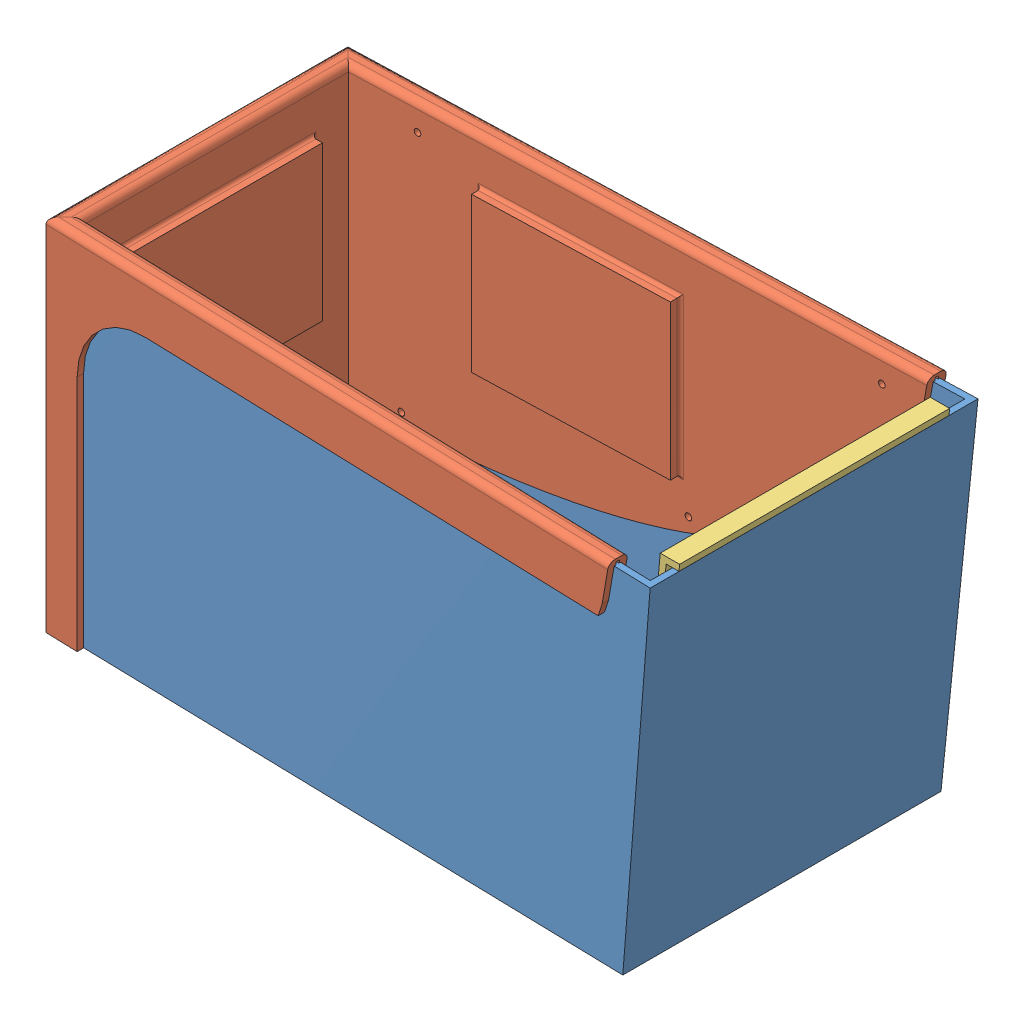
SolidWorks assembly Montagem_cesta_com_SuporteEletronica, configuration Valor predeterminado. Lengths in mm.
Overall size (1005.81 566.86 611.06).
245 component instances, 12 part files, 31 mates.
Components (placement in the parent):
- Cesta_Atualizada-1: Cesta_Atualizada [Valor predeterminado] at (-516.4663 -290.9084 0) size (950 550 510) (hidden)
- SuporteEletronica_Atualizado-1: SuporteEletronica_Atualizado [Valor predeterminado] at (-516.4663 249.0916 0) size (996.8 566.86 611.06)
- SuporteDeEletronica_Tras_Atualizado-1: SuporteDeEletronica_Tras_Atualizado [Valor predeterminado] at (-528.7672 -314.7085 0) size (75.35 498.85 420)
- Antena RFID AN610-2: Antena RFID AN610 [Valor predeterminado] at (-145.1288 78.7469 -224.7205) x (0.999502 0 -0.031563) z (0 -1 0) size (278.3 12.01 216.57)
- Antena RFID AN610-3: Antena RFID AN610 [Valor predeterminado] at (-145.2259 78.7469 224.7174) x (0.999502 0 0.031563) z (0 1 0) size (278.3 12.01 216.57)
- Antena RFID AN610-4: Antena RFID AN610 [Valor predeterminado] at (-504.4663 78.7463 1.4544) x (0 0 1) z (0 1 0) size (278.3 12.01 216.57)
- Antena RFID AN610-6: Antena RFID AN610 [Valor predeterminado] at (399.8873 88.4011 1.4544) x (0 0 1) z (-0.090536 -0.995893 0) size (278.3 12.01 216.57)
- HC-SR04-1: HC-SR04 [Default] at (-534.0577 -216.5172 151.8948) x (0.537325 0 0.843375) z (-0.843375 0 0.537325) size (45.12 25.91 17.5)
  - BoardHCSR04-1: BoardHCSR04 [Default] x (1 0 0) z (0 -1 0) size (45 1.5 20)
  - SOIC16 narrow-1: SOIC16 narrow [Default] at (-18.9903 -0.1332 0.0032) x (0 1 0) z (0 0 -1) size (10.08 6.32 2.01)
  - SOIC16 narrow-2: SOIC16 narrow [Default] at (17.2401 0.0038 0.0032) x (1 0 0) z (0 0 -1) size (10.08 6.32 2.01)
  - SOIC16 narrow-3: SOIC16 narrow [Default] at (0.0833 0.1806 0.0032) x (-1 0 0) z (0 0 -1) size (10.08 6.32 2.01)
  - Crystal Oscillator (SMD)-1: Crystal Oscillator (SMD) [Default] at (0.0865 7.1352 2.4144) x (-1 0 0) z (0 0 1) size (13.06 4.55 4.32)
  - RES 0603-33: RES 0603 [По умолчанию] at (20.0622 -5.1327 -0.45) x (-1 0 0) z (0 1 0) size (1.6 0.45 0.8)
  - RES 0603-30: RES 0603 [По умолчанию] at (20.0876 4.2055 -0.45) x (-1 0 0) z (0 1 0) size (1.6 0.45 0.8)
  - RES 0603-40: RES 0603 [По умолчанию] at (17.1224 8.2736 -0.45) x (-1 0 0) z (0 1 0) size (1.6 0.45 0.8)
  - RES 0603-43: RES 0603 [По умолчанию] at (11.9522 8.2736 -0.45) x (-1 0 0) z (0 1 0) size (1.6 0.45 0.8)
  - RES 0603-44: RES 0603 [По умолчанию] at (14.4328 8.2728 -0.45) x (-1 0 0) z (0 1 0) size (1.6 0.45 0.8)
  - RES 0603-45: RES 0603 [По умолчанию] at (11.4133 -8.8519 -0.45) x (-1 0 0) z (0 1 0) size (1.6 0.45 0.8)
  - RES 0603-46: RES 0603 [По умолчанию] at (9.1337 6.3171 -0.45) x (-1 0 0) z (0 1 0) size (1.6 0.45 0.8)
  - RES 0603-47: RES 0603 [По умолчанию] at (9.131 -5.8347 -0.45) x (-1 0 0) z (0 1 0) size (1.6 0.45 0.8)
  - RES 0603-48: RES 0603 [По умолчанию] at (9.1319 -3.7587 -0.45) x (-1 0 0) z (0 1 0) size (1.6 0.45 0.8)
  - RES 0603-49: RES 0603 [По умолчанию] at (9.1326 -1.7712 -0.45) x (-1 0 0) z (0 1 0) size (1.6 0.45 0.8)
  - RES 0603-50: RES 0603 [По умолчанию] at (-8.574 5.1664 -0.45) x (-1 0 0) z (0 1 0) size (1.6 0.45 0.8)
  - RES 0603-51: RES 0603 [По умолчанию] at (-8.6599 1.0553 -0.45) x (-1 0 0) z (0 1 0) size (1.6 0.45 0.8)
  - RES 0603-52: RES 0603 [По умолчанию] at (-8.6597 -0.8895 -0.45) x (-1 0 0) z (0 1 0) size (1.6 0.45 0.8)
  - RES 0603-53: RES 0603 [По умолчанию] at (-8.6224 -2.9356 -0.45) x (-1 0 0) z (0 1 0) size (1.6 0.45 0.8)
  - RES 0603-54: RES 0603 [По умолчанию] at (-8.6219 -5.2391 -0.45) x (-1 0 0) z (0 1 0) size (1.6 0.45 0.8)
  - RES 0603-55: RES 0603 [По умолчанию] at (-18.792 -7.4397 -0.45) x (-1 0 0) z (0 1 0) size (1.6 0.45 0.8)
  - RES 0603-56: RES 0603 [По умолчанию] at (-18.792 6.206 -0.45) x (-1 0 0) z (0 1 0) size (1.6 0.45 0.8)
  - 0603 Capacitor-2: 0603 Capacitor [Default] at (18.0116 -4.5871 0) x (0 -1 0) z (0 0 -1) size (1.6 0.84 0.84)
  - 0603 Capacitor-7: 0603 Capacitor [Default] at (15.4963 -8.9009 0) x (-1 0 0) z (0 0 -1) size (1.6 0.84 0.84)
  - 0603 Capacitor-8: 0603 Capacitor [Default] at (9.8433 0.2097 0) x (-1 0 0) z (0 0 -1) size (1.6 0.84 0.84)
  - 0603 Capacitor-17: 0603 Capacitor [Default] at (-7.8216 3.0281 0) x (-1 0 0) z (0 0 -1) size (1.6 0.84 0.84)
  - 0603 Capacitor-18: 0603 Capacitor [Default] at (18.0081 6.1516 0) x (0 -1 0) z (0 0 -1) size (1.6 0.84 0.84)
  - 0603 Capacitor-19: 0603 Capacitor [Default] at (9.8432 2.0135 0) x (-1 0 0) z (0 0 -1) size (1.6 0.84 0.84)
  - 0603 Capacitor-22: 0603 Capacitor [Default] at (9.843 3.9787 0) x (-1 0 0) z (0 0 -1) size (1.6 0.84 0.84)
  - Mesh-1: Mesh [Default] at (-7.5462 11.7833 1.7797) x (-0.435927 -0.899982 0) z (0 0 -1) size (13.88 13.88 0.41)
  - Mesh-2: Mesh [Default] at (5.988 10.9085 24.5426) x (0.558295 -0.829642 0) z (0 0 1) size (13.88 13.88 0.41)
  - PLS-4R (DS-1022-1x4)-1: PLS-4R (DS-1022-1x4) [another] at (3.81 -8.73 -2.5) x (0 -1 0) z (-1 0 0) size (8.45 7 10.16)
  - Transmitter-1: Transmitter [Default] at (0 0 1.5) x (-1 0 0) z (0 0 -1) size (42 16 14.5)
- HC-SR04-2: HC-SR04 [Default] at (-545.4669 -216.5172 115.0138) x (0.066401 0 0.997793) z (-0.997793 0 0.066401) size (45.12 25.91 17.5)
  - BoardHCSR04-1: BoardHCSR04 [Default] x (1 0 0) z (0 -1 0) size (45 1.5 20)
  - SOIC16 narrow-1: SOIC16 narrow [Default] at (-18.9903 -0.1332 0.0032) x (0 1 0) z (0 0 -1) size (10.08 6.32 2.01)
  - SOIC16 narrow-2: SOIC16 narrow [Default] at (17.2401 0.0038 0.0032) x (1 0 0) z (0 0 -1) size (10.08 6.32 2.01)
  - SOIC16 narrow-3: SOIC16 narrow [Default] at (0.0833 0.1806 0.0032) x (-1 0 0) z (0 0 -1) size (10.08 6.32 2.01)
  - Crystal Oscillator (SMD)-1: Crystal Oscillator (SMD) [Default] at (0.0865 7.1352 2.4144) x (-1 0 0) z (0 0 1) size (13.06 4.55 4.32)
  - RES 0603-33: RES 0603 [По умолчанию] at (20.0622 -5.1327 -0.45) x (-1 0 0) z (0 1 0) size (1.6 0.45 0.8)
  - RES 0603-30: RES 0603 [По умолчанию] at (20.0876 4.2055 -0.45) x (-1 0 0) z (0 1 0) size (1.6 0.45 0.8)
  - RES 0603-40: RES 0603 [По умолчанию] at (17.1224 8.2736 -0.45) x (-1 0 0) z (0 1 0) size (1.6 0.45 0.8)
  - RES 0603-43: RES 0603 [По умолчанию] at (11.9522 8.2736 -0.45) x (-1 0 0) z (0 1 0) size (1.6 0.45 0.8)
  - RES 0603-44: RES 0603 [По умолчанию] at (14.4328 8.2728 -0.45) x (-1 0 0) z (0 1 0) size (1.6 0.45 0.8)
  - RES 0603-45: RES 0603 [По умолчанию] at (11.4133 -8.8519 -0.45) x (-1 0 0) z (0 1 0) size (1.6 0.45 0.8)
  - RES 0603-46: RES 0603 [По умолчанию] at (9.1337 6.3171 -0.45) x (-1 0 0) z (0 1 0) size (1.6 0.45 0.8)
  - RES 0603-47: RES 0603 [По умолчанию] at (9.131 -5.8347 -0.45) x (-1 0 0) z (0 1 0) size (1.6 0.45 0.8)
  - RES 0603-48: RES 0603 [По умолчанию] at (9.1319 -3.7587 -0.45) x (-1 0 0) z (0 1 0) size (1.6 0.45 0.8)
  - RES 0603-49: RES 0603 [По умолчанию] at (9.1326 -1.7712 -0.45) x (-1 0 0) z (0 1 0) size (1.6 0.45 0.8)
  - RES 0603-50: RES 0603 [По умолчанию] at (-8.574 5.1664 -0.45) x (-1 0 0) z (0 1 0) size (1.6 0.45 0.8)
  - RES 0603-51: RES 0603 [По умолчанию] at (-8.6599 1.0553 -0.45) x (-1 0 0) z (0 1 0) size (1.6 0.45 0.8)
  - RES 0603-52: RES 0603 [По умолчанию] at (-8.6597 -0.8895 -0.45) x (-1 0 0) z (0 1 0) size (1.6 0.45 0.8)
  - RES 0603-53: RES 0603 [По умолчанию] at (-8.6224 -2.9356 -0.45) x (-1 0 0) z (0 1 0) size (1.6 0.45 0.8)
  - RES 0603-54: RES 0603 [По умолчанию] at (-8.6219 -5.2391 -0.45) x (-1 0 0) z (0 1 0) size (1.6 0.45 0.8)
  - RES 0603-55: RES 0603 [По умолчанию] at (-18.792 -7.4397 -0.45) x (-1 0 0) z (0 1 0) size (1.6 0.45 0.8)
  - RES 0603-56: RES 0603 [По умолчанию] at (-18.792 6.206 -0.45) x (-1 0 0) z (0 1 0) size (1.6 0.45 0.8)
  - 0603 Capacitor-2: 0603 Capacitor [Default] at (18.0116 -4.5871 0) x (0 -1 0) z (0 0 -1) size (1.6 0.84 0.84)
  - 0603 Capacitor-7: 0603 Capacitor [Default] at (15.4963 -8.9009 0) x (-1 0 0) z (0 0 -1) size (1.6 0.84 0.84)
  - 0603 Capacitor-8: 0603 Capacitor [Default] at (9.8433 0.2097 0) x (-1 0 0) z (0 0 -1) size (1.6 0.84 0.84)
  - 0603 Capacitor-17: 0603 Capacitor [Default] at (-7.8216 3.0281 0) x (-1 0 0) z (0 0 -1) size (1.6 0.84 0.84)
  - 0603 Capacitor-18: 0603 Capacitor [Default] at (18.0081 6.1516 0) x (0 -1 0) z (0 0 -1) size (1.6 0.84 0.84)
  - 0603 Capacitor-19: 0603 Capacitor [Default] at (9.8432 2.0135 0) x (-1 0 0) z (0 0 -1) size (1.6 0.84 0.84)
  - 0603 Capacitor-22: 0603 Capacitor [Default] at (9.843 3.9787 0) x (-1 0 0) z (0 0 -1) size (1.6 0.84 0.84)
  - Mesh-1: Mesh [Default] at (-7.5462 11.7833 1.7797) x (-0.435927 -0.899982 0) z (0 0 -1) size (13.88 13.88 0.41)
  - Mesh-2: Mesh [Default] at (5.988 10.9085 24.5426) x (0.558295 -0.829642 0) z (0 0 1) size (13.88 13.88 0.41)
  - PLS-4R (DS-1022-1x4)-1: PLS-4R (DS-1022-1x4) [another] at (3.81 -8.73 -2.5) x (0 -1 0) z (-1 0 0) size (8.45 7 10.16)
  - Transmitter-1: Transmitter [Default] at (0 0 1.5) x (-1 0 0) z (0 0 -1) size (42 16 14.5)
- HC-SR04-3: HC-SR04 [Default] at (-549.4828 -216.5172 57.0525) x (0.071003 0 0.997476) z (-0.997476 0 0.071003) size (45.12 25.91 17.5)
  - BoardHCSR04-1: BoardHCSR04 [Default] x (1 0 0) z (0 -1 0) size (45 1.5 20)
  - SOIC16 narrow-1: SOIC16 narrow [Default] at (-18.9903 -0.1332 0.0032) x (0 1 0) z (0 0 -1) size (10.08 6.32 2.01)
  - SOIC16 narrow-2: SOIC16 narrow [Default] at (17.2401 0.0038 0.0032) x (1 0 0) z (0 0 -1) size (10.08 6.32 2.01)
  - SOIC16 narrow-3: SOIC16 narrow [Default] at (0.0833 0.1806 0.0032) x (-1 0 0) z (0 0 -1) size (10.08 6.32 2.01)
  - Crystal Oscillator (SMD)-1: Crystal Oscillator (SMD) [Default] at (0.0865 7.1352 2.4144) x (-1 0 0) z (0 0 1) size (13.06 4.55 4.32)
  - RES 0603-33: RES 0603 [По умолчанию] at (20.0622 -5.1327 -0.45) x (-1 0 0) z (0 1 0) size (1.6 0.45 0.8)
  - RES 0603-30: RES 0603 [По умолчанию] at (20.0876 4.2055 -0.45) x (-1 0 0) z (0 1 0) size (1.6 0.45 0.8)
  - RES 0603-40: RES 0603 [По умолчанию] at (17.1224 8.2736 -0.45) x (-1 0 0) z (0 1 0) size (1.6 0.45 0.8)
  - RES 0603-43: RES 0603 [По умолчанию] at (11.9522 8.2736 -0.45) x (-1 0 0) z (0 1 0) size (1.6 0.45 0.8)
  - RES 0603-44: RES 0603 [По умолчанию] at (14.4328 8.2728 -0.45) x (-1 0 0) z (0 1 0) size (1.6 0.45 0.8)
  - RES 0603-45: RES 0603 [По умолчанию] at (11.4133 -8.8519 -0.45) x (-1 0 0) z (0 1 0) size (1.6 0.45 0.8)
  - RES 0603-46: RES 0603 [По умолчанию] at (9.1337 6.3171 -0.45) x (-1 0 0) z (0 1 0) size (1.6 0.45 0.8)
  - RES 0603-47: RES 0603 [По умолчанию] at (9.131 -5.8347 -0.45) x (-1 0 0) z (0 1 0) size (1.6 0.45 0.8)
  - RES 0603-48: RES 0603 [По умолчанию] at (9.1319 -3.7587 -0.45) x (-1 0 0) z (0 1 0) size (1.6 0.45 0.8)
  - RES 0603-49: RES 0603 [По умолчанию] at (9.1326 -1.7712 -0.45) x (-1 0 0) z (0 1 0) size (1.6 0.45 0.8)
  - RES 0603-50: RES 0603 [По умолчанию] at (-8.574 5.1664 -0.45) x (-1 0 0) z (0 1 0) size (1.6 0.45 0.8)
  - RES 0603-51: RES 0603 [По умолчанию] at (-8.6599 1.0553 -0.45) x (-1 0 0) z (0 1 0) size (1.6 0.45 0.8)
  - RES 0603-52: RES 0603 [По умолчанию] at (-8.6597 -0.8895 -0.45) x (-1 0 0) z (0 1 0) size (1.6 0.45 0.8)
  - RES 0603-53: RES 0603 [По умолчанию] at (-8.6224 -2.9356 -0.45) x (-1 0 0) z (0 1 0) size (1.6 0.45 0.8)
  - RES 0603-54: RES 0603 [По умолчанию] at (-8.6219 -5.2391 -0.45) x (-1 0 0) z (0 1 0) size (1.6 0.45 0.8)
  - RES 0603-55: RES 0603 [По умолчанию] at (-18.792 -7.4397 -0.45) x (-1 0 0) z (0 1 0) size (1.6 0.45 0.8)
  - RES 0603-56: RES 0603 [По умолчанию] at (-18.792 6.206 -0.45) x (-1 0 0) z (0 1 0) size (1.6 0.45 0.8)
  - 0603 Capacitor-2: 0603 Capacitor [Default] at (18.0116 -4.5871 0) x (0 -1 0) z (0 0 -1) size (1.6 0.84 0.84)
  - 0603 Capacitor-7: 0603 Capacitor [Default] at (15.4963 -8.9009 0) x (-1 0 0) z (0 0 -1) size (1.6 0.84 0.84)
  - 0603 Capacitor-8: 0603 Capacitor [Default] at (9.8433 0.2097 0) x (-1 0 0) z (0 0 -1) size (1.6 0.84 0.84)
  - 0603 Capacitor-17: 0603 Capacitor [Default] at (-7.8216 3.0281 0) x (-1 0 0) z (0 0 -1) size (1.6 0.84 0.84)
  - 0603 Capacitor-18: 0603 Capacitor [Default] at (18.0081 6.1516 0) x (0 -1 0) z (0 0 -1) size (1.6 0.84 0.84)
  - 0603 Capacitor-19: 0603 Capacitor [Default] at (9.8432 2.0135 0) x (-1 0 0) z (0 0 -1) size (1.6 0.84 0.84)
  - 0603 Capacitor-22: 0603 Capacitor [Default] at (9.843 3.9787 0) x (-1 0 0) z (0 0 -1) size (1.6 0.84 0.84)
  - Mesh-1: Mesh [Default] at (-7.5462 11.7833 1.7797) x (-0.435927 -0.899982 0) z (0 0 -1) size (13.88 13.88 0.41)
  - Mesh-2: Mesh [Default] at (5.988 10.9085 24.5426) x (0.558295 -0.829642 0) z (0 0 1) size (13.88 13.88 0.41)
  - PLS-4R (DS-1022-1x4)-1: PLS-4R (DS-1022-1x4) [another] at (3.81 -8.73 -2.5) x (0 -1 0) z (-1 0 0) size (8.45 7 10.16)
  - Transmitter-1: Transmitter [Default] at (0 0 1.5) x (-1 0 0) z (0 0 -1) size (42 16 14.5)
- HC-SR04-4: HC-SR04 [Default] at (-551.8136 -216.5172 -0.4786) x (0 0 1) z (-1 0 0) size (45.12 25.91 17.5)
  - BoardHCSR04-1: BoardHCSR04 [Default] x (1 0 0) z (0 -1 0) size (45 1.5 20)
  - SOIC16 narrow-1: SOIC16 narrow [Default] at (-18.9903 -0.1332 0.0032) x (0 1 0) z (0 0 -1) size (10.08 6.32 2.01)
  - SOIC16 narrow-2: SOIC16 narrow [Default] at (17.2401 0.0038 0.0032) x (1 0 0) z (0 0 -1) size (10.08 6.32 2.01)
  - SOIC16 narrow-3: SOIC16 narrow [Default] at (0.0833 0.1806 0.0032) x (-1 0 0) z (0 0 -1) size (10.08 6.32 2.01)
  - Crystal Oscillator (SMD)-1: Crystal Oscillator (SMD) [Default] at (0.0865 7.1352 2.4144) x (-1 0 0) z (0 0 1) size (13.06 4.55 4.32)
  - RES 0603-33: RES 0603 [По умолчанию] at (20.0622 -5.1327 -0.45) x (-1 0 0) z (0 1 0) size (1.6 0.45 0.8)
  - RES 0603-30: RES 0603 [По умолчанию] at (20.0876 4.2055 -0.45) x (-1 0 0) z (0 1 0) size (1.6 0.45 0.8)
  - RES 0603-40: RES 0603 [По умолчанию] at (17.1224 8.2736 -0.45) x (-1 0 0) z (0 1 0) size (1.6 0.45 0.8)
  - RES 0603-43: RES 0603 [По умолчанию] at (11.9522 8.2736 -0.45) x (-1 0 0) z (0 1 0) size (1.6 0.45 0.8)
  - RES 0603-44: RES 0603 [По умолчанию] at (14.4328 8.2728 -0.45) x (-1 0 0) z (0 1 0) size (1.6 0.45 0.8)
  - RES 0603-45: RES 0603 [По умолчанию] at (11.4133 -8.8519 -0.45) x (-1 0 0) z (0 1 0) size (1.6 0.45 0.8)
  - RES 0603-46: RES 0603 [По умолчанию] at (9.1337 6.3171 -0.45) x (-1 0 0) z (0 1 0) size (1.6 0.45 0.8)
  - RES 0603-47: RES 0603 [По умолчанию] at (9.131 -5.8347 -0.45) x (-1 0 0) z (0 1 0) size (1.6 0.45 0.8)
  - RES 0603-48: RES 0603 [По умолчанию] at (9.1319 -3.7587 -0.45) x (-1 0 0) z (0 1 0) size (1.6 0.45 0.8)
  - RES 0603-49: RES 0603 [По умолчанию] at (9.1326 -1.7712 -0.45) x (-1 0 0) z (0 1 0) size (1.6 0.45 0.8)
  - RES 0603-50: RES 0603 [По умолчанию] at (-8.574 5.1664 -0.45) x (-1 0 0) z (0 1 0) size (1.6 0.45 0.8)
  - RES 0603-51: RES 0603 [По умолчанию] at (-8.6599 1.0553 -0.45) x (-1 0 0) z (0 1 0) size (1.6 0.45 0.8)
  - RES 0603-52: RES 0603 [По умолчанию] at (-8.6597 -0.8895 -0.45) x (-1 0 0) z (0 1 0) size (1.6 0.45 0.8)
  - RES 0603-53: RES 0603 [По умолчанию] at (-8.6224 -2.9356 -0.45) x (-1 0 0) z (0 1 0) size (1.6 0.45 0.8)
  - RES 0603-54: RES 0603 [По умолчанию] at (-8.6219 -5.2391 -0.45) x (-1 0 0) z (0 1 0) size (1.6 0.45 0.8)
  - RES 0603-55: RES 0603 [По умолчанию] at (-18.792 -7.4397 -0.45) x (-1 0 0) z (0 1 0) size (1.6 0.45 0.8)
  - RES 0603-56: RES 0603 [По умолчанию] at (-18.792 6.206 -0.45) x (-1 0 0) z (0 1 0) size (1.6 0.45 0.8)
  - 0603 Capacitor-2: 0603 Capacitor [Default] at (18.0116 -4.5871 0) x (0 -1 0) z (0 0 -1) size (1.6 0.84 0.84)
  - 0603 Capacitor-7: 0603 Capacitor [Default] at (15.4963 -8.9009 0) x (-1 0 0) z (0 0 -1) size (1.6 0.84 0.84)
  - 0603 Capacitor-8: 0603 Capacitor [Default] at (9.8433 0.2097 0) x (-1 0 0) z (0 0 -1) size (1.6 0.84 0.84)
  - 0603 Capacitor-17: 0603 Capacitor [Default] at (-7.8216 3.0281 0) x (-1 0 0) z (0 0 -1) size (1.6 0.84 0.84)
  - 0603 Capacitor-18: 0603 Capacitor [Default] at (18.0081 6.1516 0) x (0 -1 0) z (0 0 -1) size (1.6 0.84 0.84)
  - 0603 Capacitor-19: 0603 Capacitor [Default] at (9.8432 2.0135 0) x (-1 0 0) z (0 0 -1) size (1.6 0.84 0.84)
  - 0603 Capacitor-22: 0603 Capacitor [Default] at (9.843 3.9787 0) x (-1 0 0) z (0 0 -1) size (1.6 0.84 0.84)
  - Mesh-1: Mesh [Default] at (-7.5462 11.7833 1.7797) x (-0.435927 -0.899982 0) z (0 0 -1) size (13.88 13.88 0.41)
  - Mesh-2: Mesh [Default] at (5.988 10.9085 24.5426) x (0.558295 -0.829642 0) z (0 0 1) size (13.88 13.88 0.41)
  - PLS-4R (DS-1022-1x4)-1: PLS-4R (DS-1022-1x4) [another] at (3.81 -8.73 -2.5) x (0 -1 0) z (-1 0 0) size (8.45 7 10.16)
  - Transmitter-1: Transmitter [Default] at (0 0 1.5) x (-1 0 0) z (0 0 -1) size (42 16 14.5)
- HC-SR04-5: HC-SR04 [Default] at (-549.4139 -216.5172 -58.0073) x (-0.071003 0 0.997476) z (-0.997476 0 -0.071003) size (45.12 25.91 17.5)
  - BoardHCSR04-1: BoardHCSR04 [Default] x (1 0 0) z (0 -1 0) size (45 1.5 20)
  - SOIC16 narrow-1: SOIC16 narrow [Default] at (-18.9903 -0.1332 0.0032) x (0 1 0) z (0 0 -1) size (10.08 6.32 2.01)
  - SOIC16 narrow-2: SOIC16 narrow [Default] at (17.2401 0.0038 0.0032) x (1 0 0) z (0 0 -1) size (10.08 6.32 2.01)
  - SOIC16 narrow-3: SOIC16 narrow [Default] at (0.0833 0.1806 0.0032) x (-1 0 0) z (0 0 -1) size (10.08 6.32 2.01)
  - Crystal Oscillator (SMD)-1: Crystal Oscillator (SMD) [Default] at (0.0865 7.1352 2.4144) x (-1 0 0) z (0 0 1) size (13.06 4.55 4.32)
  - RES 0603-33: RES 0603 [По умолчанию] at (20.0622 -5.1327 -0.45) x (-1 0 0) z (0 1 0) size (1.6 0.45 0.8)
  - RES 0603-30: RES 0603 [По умолчанию] at (20.0876 4.2055 -0.45) x (-1 0 0) z (0 1 0) size (1.6 0.45 0.8)
  - RES 0603-40: RES 0603 [По умолчанию] at (17.1224 8.2736 -0.45) x (-1 0 0) z (0 1 0) size (1.6 0.45 0.8)
  - RES 0603-43: RES 0603 [По умолчанию] at (11.9522 8.2736 -0.45) x (-1 0 0) z (0 1 0) size (1.6 0.45 0.8)
  - RES 0603-44: RES 0603 [По умолчанию] at (14.4328 8.2728 -0.45) x (-1 0 0) z (0 1 0) size (1.6 0.45 0.8)
  - RES 0603-45: RES 0603 [По умолчанию] at (11.4133 -8.8519 -0.45) x (-1 0 0) z (0 1 0) size (1.6 0.45 0.8)
  - RES 0603-46: RES 0603 [По умолчанию] at (9.1337 6.3171 -0.45) x (-1 0 0) z (0 1 0) size (1.6 0.45 0.8)
  - RES 0603-47: RES 0603 [По умолчанию] at (9.131 -5.8347 -0.45) x (-1 0 0) z (0 1 0) size (1.6 0.45 0.8)
  - RES 0603-48: RES 0603 [По умолчанию] at (9.1319 -3.7587 -0.45) x (-1 0 0) z (0 1 0) size (1.6 0.45 0.8)
  - RES 0603-49: RES 0603 [По умолчанию] at (9.1326 -1.7712 -0.45) x (-1 0 0) z (0 1 0) size (1.6 0.45 0.8)
  - RES 0603-50: RES 0603 [По умолчанию] at (-8.574 5.1664 -0.45) x (-1 0 0) z (0 1 0) size (1.6 0.45 0.8)
  - RES 0603-51: RES 0603 [По умолчанию] at (-8.6599 1.0553 -0.45) x (-1 0 0) z (0 1 0) size (1.6 0.45 0.8)
  - RES 0603-52: RES 0603 [По умолчанию] at (-8.6597 -0.8895 -0.45) x (-1 0 0) z (0 1 0) size (1.6 0.45 0.8)
  - RES 0603-53: RES 0603 [По умолчанию] at (-8.6224 -2.9356 -0.45) x (-1 0 0) z (0 1 0) size (1.6 0.45 0.8)
  - RES 0603-54: RES 0603 [По умолчанию] at (-8.6219 -5.2391 -0.45) x (-1 0 0) z (0 1 0) size (1.6 0.45 0.8)
  - RES 0603-55: RES 0603 [По умолчанию] at (-18.792 -7.4397 -0.45) x (-1 0 0) z (0 1 0) size (1.6 0.45 0.8)
  - RES 0603-56: RES 0603 [По умолчанию] at (-18.792 6.206 -0.45) x (-1 0 0) z (0 1 0) size (1.6 0.45 0.8)
  - 0603 Capacitor-2: 0603 Capacitor [Default] at (18.0116 -4.5871 0) x (0 -1 0) z (0 0 -1) size (1.6 0.84 0.84)
  - 0603 Capacitor-7: 0603 Capacitor [Default] at (15.4963 -8.9009 0) x (-1 0 0) z (0 0 -1) size (1.6 0.84 0.84)
  - 0603 Capacitor-8: 0603 Capacitor [Default] at (9.8433 0.2097 0) x (-1 0 0) z (0 0 -1) size (1.6 0.84 0.84)
  - 0603 Capacitor-17: 0603 Capacitor [Default] at (-7.8216 3.0281 0) x (-1 0 0) z (0 0 -1) size (1.6 0.84 0.84)
  - 0603 Capacitor-18: 0603 Capacitor [Default] at (18.0081 6.1516 0) x (0 -1 0) z (0 0 -1) size (1.6 0.84 0.84)
  - 0603 Capacitor-19: 0603 Capacitor [Default] at (9.8432 2.0135 0) x (-1 0 0) z (0 0 -1) size (1.6 0.84 0.84)
  - 0603 Capacitor-22: 0603 Capacitor [Default] at (9.843 3.9787 0) x (-1 0 0) z (0 0 -1) size (1.6 0.84 0.84)
  - Mesh-1: Mesh [Default] at (-7.5462 11.7833 1.7797) x (-0.435927 -0.899982 0) z (0 0 -1) size (13.88 13.88 0.41)
  - Mesh-2: Mesh [Default] at (5.988 10.9085 24.5426) x (0.558295 -0.829642 0) z (0 0 1) size (13.88 13.88 0.41)
  - PLS-4R (DS-1022-1x4)-1: PLS-4R (DS-1022-1x4) [another] at (3.81 -8.73 -2.5) x (0 -1 0) z (-1 0 0) size (8.45 7 10.16)
  - Transmitter-1: Transmitter [Default] at (0 0 1.5) x (-1 0 0) z (0 0 -1) size (42 16 14.5)
- HC-SR04-6: HC-SR04 [Default] at (-545.3183 -216.5172 -117.2336) x (-0.066401 0 0.997793) z (-0.997793 0 -0.066401) size (45.12 25.91 17.5)
  - BoardHCSR04-1: BoardHCSR04 [Default] x (1 0 0) z (0 -1 0) size (45 1.5 20)
  - SOIC16 narrow-1: SOIC16 narrow [Default] at (-18.9903 -0.1332 0.0032) x (0 1 0) z (0 0 -1) size (10.08 6.32 2.01)
  - SOIC16 narrow-2: SOIC16 narrow [Default] at (17.2401 0.0038 0.0032) x (1 0 0) z (0 0 -1) size (10.08 6.32 2.01)
  - SOIC16 narrow-3: SOIC16 narrow [Default] at (0.0833 0.1806 0.0032) x (-1 0 0) z (0 0 -1) size (10.08 6.32 2.01)
  - Crystal Oscillator (SMD)-1: Crystal Oscillator (SMD) [Default] at (0.0865 7.1352 2.4144) x (-1 0 0) z (0 0 1) size (13.06 4.55 4.32)
  - RES 0603-33: RES 0603 [По умолчанию] at (20.0622 -5.1327 -0.45) x (-1 0 0) z (0 1 0) size (1.6 0.45 0.8)
  - RES 0603-30: RES 0603 [По умолчанию] at (20.0876 4.2055 -0.45) x (-1 0 0) z (0 1 0) size (1.6 0.45 0.8)
  - RES 0603-40: RES 0603 [По умолчанию] at (17.1224 8.2736 -0.45) x (-1 0 0) z (0 1 0) size (1.6 0.45 0.8)
  - RES 0603-43: RES 0603 [По умолчанию] at (11.9522 8.2736 -0.45) x (-1 0 0) z (0 1 0) size (1.6 0.45 0.8)
  - RES 0603-44: RES 0603 [По умолчанию] at (14.4328 8.2728 -0.45) x (-1 0 0) z (0 1 0) size (1.6 0.45 0.8)
  - RES 0603-45: RES 0603 [По умолчанию] at (11.4133 -8.8519 -0.45) x (-1 0 0) z (0 1 0) size (1.6 0.45 0.8)
  - RES 0603-46: RES 0603 [По умолчанию] at (9.1337 6.3171 -0.45) x (-1 0 0) z (0 1 0) size (1.6 0.45 0.8)
  - RES 0603-47: RES 0603 [По умолчанию] at (9.131 -5.8347 -0.45) x (-1 0 0) z (0 1 0) size (1.6 0.45 0.8)
  - RES 0603-48: RES 0603 [По умолчанию] at (9.1319 -3.7587 -0.45) x (-1 0 0) z (0 1 0) size (1.6 0.45 0.8)
  - RES 0603-49: RES 0603 [По умолчанию] at (9.1326 -1.7712 -0.45) x (-1 0 0) z (0 1 0) size (1.6 0.45 0.8)
  - RES 0603-50: RES 0603 [По умолчанию] at (-8.574 5.1664 -0.45) x (-1 0 0) z (0 1 0) size (1.6 0.45 0.8)
  - RES 0603-51: RES 0603 [По умолчанию] at (-8.6599 1.0553 -0.45) x (-1 0 0) z (0 1 0) size (1.6 0.45 0.8)
  - RES 0603-52: RES 0603 [По умолчанию] at (-8.6597 -0.8895 -0.45) x (-1 0 0) z (0 1 0) size (1.6 0.45 0.8)
  - RES 0603-53: RES 0603 [По умолчанию] at (-8.6224 -2.9356 -0.45) x (-1 0 0) z (0 1 0) size (1.6 0.45 0.8)
  - RES 0603-54: RES 0603 [По умолчанию] at (-8.6219 -5.2391 -0.45) x (-1 0 0) z (0 1 0) size (1.6 0.45 0.8)
  - RES 0603-55: RES 0603 [По умолчанию] at (-18.792 -7.4397 -0.45) x (-1 0 0) z (0 1 0) size (1.6 0.45 0.8)
  - RES 0603-56: RES 0603 [По умолчанию] at (-18.792 6.206 -0.45) x (-1 0 0) z (0 1 0) size (1.6 0.45 0.8)
  - 0603 Capacitor-2: 0603 Capacitor [Default] at (18.0116 -4.5871 0) x (0 -1 0) z (0 0 -1) size (1.6 0.84 0.84)
  - 0603 Capacitor-7: 0603 Capacitor [Default] at (15.4963 -8.9009 0) x (-1 0 0) z (0 0 -1) size (1.6 0.84 0.84)
  - 0603 Capacitor-8: 0603 Capacitor [Default] at (9.8433 0.2097 0) x (-1 0 0) z (0 0 -1) size (1.6 0.84 0.84)
  - 0603 Capacitor-17: 0603 Capacitor [Default] at (-7.8216 3.0281 0) x (-1 0 0) z (0 0 -1) size (1.6 0.84 0.84)
  - 0603 Capacitor-18: 0603 Capacitor [Default] at (18.0081 6.1516 0) x (0 -1 0) z (0 0 -1) size (1.6 0.84 0.84)
  - 0603 Capacitor-19: 0603 Capacitor [Default] at (9.8432 2.0135 0) x (-1 0 0) z (0 0 -1) size (1.6 0.84 0.84)
  - 0603 Capacitor-22: 0603 Capacitor [Default] at (9.843 3.9787 0) x (-1 0 0) z (0 0 -1) size (1.6 0.84 0.84)
  - Mesh-1: Mesh [Default] at (-7.5462 11.7833 1.7797) x (-0.435927 -0.899982 0) z (0 0 -1) size (13.88 13.88 0.41)
  - Mesh-2: Mesh [Default] at (5.988 10.9085 24.5426) x (0.558295 -0.829642 0) z (0 0 1) size (13.88 13.88 0.41)
  - PLS-4R (DS-1022-1x4)-1: PLS-4R (DS-1022-1x4) [another] at (3.81 -8.73 -2.5) x (0 -1 0) z (-1 0 0) size (8.45 7 10.16)
  - Transmitter-1: Transmitter [Default] at (0 0 1.5) x (-1 0 0) z (0 0 -1) size (42 16 14.5)
- HC-SR04-7: HC-SR04 [Default] at (-532.8551 -216.5172 -153.7689) x (-0.537325 0 0.843375) z (-0.843375 0 -0.537325) size (45.12 25.91 17.5)
  - BoardHCSR04-1: BoardHCSR04 [Default] x (1 0 0) z (0 -1 0) size (45 1.5 20)
  - SOIC16 narrow-1: SOIC16 narrow [Default] at (-18.9903 -0.1332 0.0032) x (0 1 0) z (0 0 -1) size (10.08 6.32 2.01)
  - SOIC16 narrow-2: SOIC16 narrow [Default] at (17.2401 0.0038 0.0032) x (1 0 0) z (0 0 -1) size (10.08 6.32 2.01)
  - SOIC16 narrow-3: SOIC16 narrow [Default] at (0.0833 0.1806 0.0032) x (-1 0 0) z (0 0 -1) size (10.08 6.32 2.01)
  - Crystal Oscillator (SMD)-1: Crystal Oscillator (SMD) [Default] at (0.0865 7.1352 2.4144) x (-1 0 0) z (0 0 1) size (13.06 4.55 4.32)
  - RES 0603-33: RES 0603 [По умолчанию] at (20.0622 -5.1327 -0.45) x (-1 0 0) z (0 1 0) size (1.6 0.45 0.8)
  - RES 0603-30: RES 0603 [По умолчанию] at (20.0876 4.2055 -0.45) x (-1 0 0) z (0 1 0) size (1.6 0.45 0.8)
  - RES 0603-40: RES 0603 [По умолчанию] at (17.1224 8.2736 -0.45) x (-1 0 0) z (0 1 0) size (1.6 0.45 0.8)
  - RES 0603-43: RES 0603 [По умолчанию] at (11.9522 8.2736 -0.45) x (-1 0 0) z (0 1 0) size (1.6 0.45 0.8)
  - RES 0603-44: RES 0603 [По умолчанию] at (14.4328 8.2728 -0.45) x (-1 0 0) z (0 1 0) size (1.6 0.45 0.8)
  - RES 0603-45: RES 0603 [По умолчанию] at (11.4133 -8.8519 -0.45) x (-1 0 0) z (0 1 0) size (1.6 0.45 0.8)
  - RES 0603-46: RES 0603 [По умолчанию] at (9.1337 6.3171 -0.45) x (-1 0 0) z (0 1 0) size (1.6 0.45 0.8)
  - RES 0603-47: RES 0603 [По умолчанию] at (9.131 -5.8347 -0.45) x (-1 0 0) z (0 1 0) size (1.6 0.45 0.8)
  - RES 0603-48: RES 0603 [По умолчанию] at (9.1319 -3.7587 -0.45) x (-1 0 0) z (0 1 0) size (1.6 0.45 0.8)
  - RES 0603-49: RES 0603 [По умолчанию] at (9.1326 -1.7712 -0.45) x (-1 0 0) z (0 1 0) size (1.6 0.45 0.8)
  - RES 0603-50: RES 0603 [По умолчанию] at (-8.574 5.1664 -0.45) x (-1 0 0) z (0 1 0) size (1.6 0.45 0.8)
  - RES 0603-51: RES 0603 [По умолчанию] at (-8.6599 1.0553 -0.45) x (-1 0 0) z (0 1 0) size (1.6 0.45 0.8)
  - RES 0603-52: RES 0603 [По умолчанию] at (-8.6597 -0.8895 -0.45) x (-1 0 0) z (0 1 0) size (1.6 0.45 0.8)
  - RES 0603-53: RES 0603 [По умолчанию] at (-8.6224 -2.9356 -0.45) x (-1 0 0) z (0 1 0) size (1.6 0.45 0.8)
  - RES 0603-54: RES 0603 [По умолчанию] at (-8.6219 -5.2391 -0.45) x (-1 0 0) z (0 1 0) size (1.6 0.45 0.8)
  - RES 0603-55: RES 0603 [По умолчанию] at (-18.792 -7.4397 -0.45) x (-1 0 0) z (0 1 0) size (1.6 0.45 0.8)
  - RES 0603-56: RES 0603 [По умолчанию] at (-18.792 6.206 -0.45) x (-1 0 0) z (0 1 0) size (1.6 0.45 0.8)
  - 0603 Capacitor-2: 0603 Capacitor [Default] at (18.0116 -4.5871 0) x (0 -1 0) z (0 0 -1) size (1.6 0.84 0.84)
  - 0603 Capacitor-7: 0603 Capacitor [Default] at (15.4963 -8.9009 0) x (-1 0 0) z (0 0 -1) size (1.6 0.84 0.84)
  - 0603 Capacitor-8: 0603 Capacitor [Default] at (9.8433 0.2097 0) x (-1 0 0) z (0 0 -1) size (1.6 0.84 0.84)
  - 0603 Capacitor-17: 0603 Capacitor [Default] at (-7.8216 3.0281 0) x (-1 0 0) z (0 0 -1) size (1.6 0.84 0.84)
  - 0603 Capacitor-18: 0603 Capacitor [Default] at (18.0081 6.1516 0) x (0 -1 0) z (0 0 -1) size (1.6 0.84 0.84)
  - 0603 Capacitor-19: 0603 Capacitor [Default] at (9.8432 2.0135 0) x (-1 0 0) z (0 0 -1) size (1.6 0.84 0.84)
  - 0603 Capacitor-22: 0603 Capacitor [Default] at (9.843 3.9787 0) x (-1 0 0) z (0 0 -1) size (1.6 0.84 0.84)
  - Mesh-1: Mesh [Default] at (-7.5462 11.7833 1.7797) x (-0.435927 -0.899982 0) z (0 0 -1) size (13.88 13.88 0.41)
  - Mesh-2: Mesh [Default] at (5.988 10.9085 24.5426) x (0.558295 -0.829642 0) z (0 0 1) size (13.88 13.88 0.41)
  - PLS-4R (DS-1022-1x4)-1: PLS-4R (DS-1022-1x4) [another] at (3.81 -8.73 -2.5) x (0 -1 0) z (-1 0 0) size (8.45 7 10.16)
  - Transmitter-1: Transmitter [Default] at (0 0 1.5) x (-1 0 0) z (0 0 -1) size (42 16 14.5)
Mates (geometry in assembly coordinates):
- Coincidente6: coincident anti-aligned: plane of Cesta_Atualizada-1 through (-516.4663 -290.9084 0) normal (-1 0 0); plane of SuporteEletronica_Atualizado-1 through (-516.4663 189.0916 235.7581) normal (1 0 0)
- Coincidente7: coincident anti-aligned: plane of Cesta_Atualizada-1 through (-516.4663 259.0916 0) normal (0 1 0); plane of SuporteEletronica_Atualizado-1 through (433.5337 259.0916 255) normal (0 -1 0)
- Tangente5: tangent: plane of assembly; face of Cesta_Atualizada-1; plane of SuporteEletronica_Atualizado-1 through (-527.219 189.0916 -224.6604) normal (0.031563 0 0.999502)
- Coincidente8: coincident anti-aligned: plane of Cesta_Atualizada-1 through (-516.4663 259.0916 0) normal (0 1 0); plane of SuporteDeEletronica_Tras_Atualizado-1 through (413.3964 259.0916 -255) normal (0 -1 0)
- Coincidente16: coincident aligned: line of Cesta_Atualizada-1 through (950 433.5337 269.0916) axis (0 -1 0); line of SuporteDeEletronica_Tras_Atualizado-1 through (434.3467 269.0916 0) axis (-1 0 0)
- Tangent1: tangent: plane of SuporteEletronica_Atualizado-1 through (-522.8069 249.0916 -200.7878) normal (-0.031563 0 -0.999502); edge_curve of ?
- Tangent2: tangent anti-aligned: cylinder of SuporteEletronica_Atualizado-1 through (-19.9057 174.7416 -228.6749) axis (0.031563 0 0.999502) radius 4.5; edge_curve of ?
- Tangent3: tangent anti-aligned: plane of SuporteEletronica_Atualizado-1 through (-522.8069 249.0916 -200.7878) normal (-0.031563 0 -0.999502); edge_curve of Antena RFID AN610-2
- Tangent4: tangent anti-aligned: cylinder of SuporteEletronica_Atualizado-1 through (-273.2594 -17.2484 -220.6742) axis (0.031563 0 0.999502) radius 4.5; edge_curve of Antena RFID AN610-2
- Tangent5: tangent anti-aligned: plane of SuporteEletronica_Atualizado-1 through (-522.8069 249.0916 200.7878) normal (-0.031563 0 0.999502); edge_curve of Antena RFID AN610-3
- Tangent6: tangent anti-aligned: cylinder of SuporteEletronica_Atualizado-1 through (-19.9057 -17.2484 228.6749) axis (0.031563 0 -0.999502) radius 4.5; edge_curve of Antena RFID AN610-3
- Tangent7: tangent anti-aligned: plane of SuporteEletronica_Atualizado-1 through (-492.4663 249.0916 0) normal (-1 0 0); edge_curve of Antena RFID AN610-4
- Tangent8: tangent anti-aligned: cylinder of SuporteEletronica_Atualizado-1 through (-504.4663 174.7416 -126.74) axis (1 0 0) radius 4.5; edge_curve of Antena RFID AN610-4
- Tangent9: tangent anti-aligned: plane of SuporteDeEletronica_Tras_Atualizado-1 through (343.9787 -394.0491 0) normal (0.995893 -0.090536 0); edge_curve of ?
- Tangent10: tangent anti-aligned: cylinder of SuporteDeEletronica_Tras_Atualizado-1 through (408.5783 184.0016 126.74) axis (-0.995893 0.090536 0) radius 4.5; edge_curve of ?
- Tangent12: tangent anti-aligned: plane of SuporteDeEletronica_Tras_Atualizado-1 through (343.9787 -394.0491 0) normal (0.995893 -0.090536 0); edge_curve of Antena RFID AN610-6
- Tangent14: tangent anti-aligned: cylinder of SuporteDeEletronica_Tras_Atualizado-1 through (391.1963 -7.2 -126.74) axis (-0.995893 0.090536 0) radius 4.5; edge_curve of Antena RFID AN610-6
- Concentric1: concentric aligned: cylinder of SuporteEletronica_Atualizado-1 through (-571.752 -211.9084 192.5818) axis (0.843375 0 -0.537325) radius 8; cylinder of HC-SR04-1/HC-SR04.stp-1/Transducer.stp-1 through (-538.017 -211.9084 171.0888) axis (0.843375 0 -0.537325) radius 7.9502
- Coincident1: coincident anti-aligned: circle of SuporteEletronica_Atualizado-1; plane of HC-SR04-1/HC-SR04.stp-1/Transducer.stp-1 through (-538.017 -211.9084 171.0888) normal (-0.843375 0 0.537325)
- Concentric2: concentric aligned: cylinder of SuporteEletronica_Atualizado-1 through (-580.355 -211.9084 131.427) axis (0.997793 0 -0.066401) radius 8; cylinder of HC-SR04-2/HC-SR04.stp-1/Transducer.stp-1 through (-558.1558 -211.9084 129.9497) axis (0.997793 0 -0.066401) radius 7.9502
- Coincident2: coincident anti-aligned: circle of SuporteEletronica_Atualizado-1; plane of HC-SR04-2/HC-SR04.stp-1/Transducer.stp-1 through (-558.1558 -211.9084 129.9497) normal (-0.997793 0 0.066401)
- Concentric3: concentric aligned: cylinder of SuporteEletronica_Atualizado-1 through (-585.0844 -211.9084 73.6827) axis (0.997476 0 -0.071003) radius 8; cylinder of HC-SR04-3/HC-SR04.stp-1/Transducer.stp-1 through (-562.1026 -211.9084 72.0467) axis (0.997476 0 -0.071003) radius 7.9502
- Coincident3: coincident anti-aligned: circle of SuporteEletronica_Atualizado-1; plane of HC-SR04-3/HC-SR04.stp-1/Transducer.stp-1 through (-562.1026 -211.9084 72.0467) normal (-0.997476 0 0.071003)
- Concentric4: concentric aligned: cylinder of SuporteEletronica_Atualizado-1 through (-571.4663 -211.9084 13.5817) axis (1 0 0) radius 8; cylinder of HC-SR04-4/HC-SR04.stp-1/Transducer.stp-1 through (-565.4663 -211.9084 13.5817) axis (1 0 0) radius 7.9502
- Coincident4: coincident anti-aligned: circle of SuporteEletronica_Atualizado-1; plane of HC-SR04-4/HC-SR04.stp-1/Transducer.stp-1 through (-565.4663 -211.9084 13.5817) normal (-1 0 0)
- Concentric5: concentric aligned: cylinder of SuporteEletronica_Atualizado-1 through (-587.0131 -211.9084 -46.5878) axis (0.997476 0 0.071003) radius 8; cylinder of HC-SR04-5/HC-SR04.stp-1/Transducer.stp-1 through (-564.0304 -211.9084 -44.9518) axis (0.997476 0 0.071003) radius 7.9502
- Coincident5: coincident anti-aligned: circle of SuporteEletronica_Atualizado-1; plane of HC-SR04-5/HC-SR04.stp-1/Transducer.stp-1 through (-564.0304 -211.9084 -44.9518) normal (-0.997476 0 -0.071003)
- Concentric6: concentric aligned: cylinder of SuporteEletronica_Atualizado-1 through (-580.3559 -211.9084 -131.4136) axis (0.997793 0 0.066401) radius 8; cylinder of HC-SR04-6/HC-SR04.stp-1/Transducer.stp-1 through (-558.1558 -211.9084 -129.9363) axis (0.997793 0 0.066401) radius 7.9502
- Coincident6: coincident anti-aligned: circle of SuporteEletronica_Atualizado-1; plane of HC-SR04-6/HC-SR04.stp-1/Transducer.stp-1 through (-558.1558 -211.9084 -129.9363) normal (-0.997793 0 -0.066401)
- Concentric7: concentric aligned: cylinder of SuporteEletronica_Atualizado-1 through (-604.3701 -211.9084 -213.3498) axis (0.843375 0 0.537325) radius 8; cylinder of HC-SR04-7/HC-SR04.stp-1/Transducer.stp-1 through (-538.017 -211.9084 -171.0754) axis (0.843375 0 0.537325) radius 7.9502
- Coincident7: coincident anti-aligned: circle of SuporteEletronica_Atualizado-1; plane of HC-SR04-7/HC-SR04.stp-1/Transducer.stp-1 through (-538.017 -211.9084 -171.0754) normal (-0.843375 0 -0.537325)
